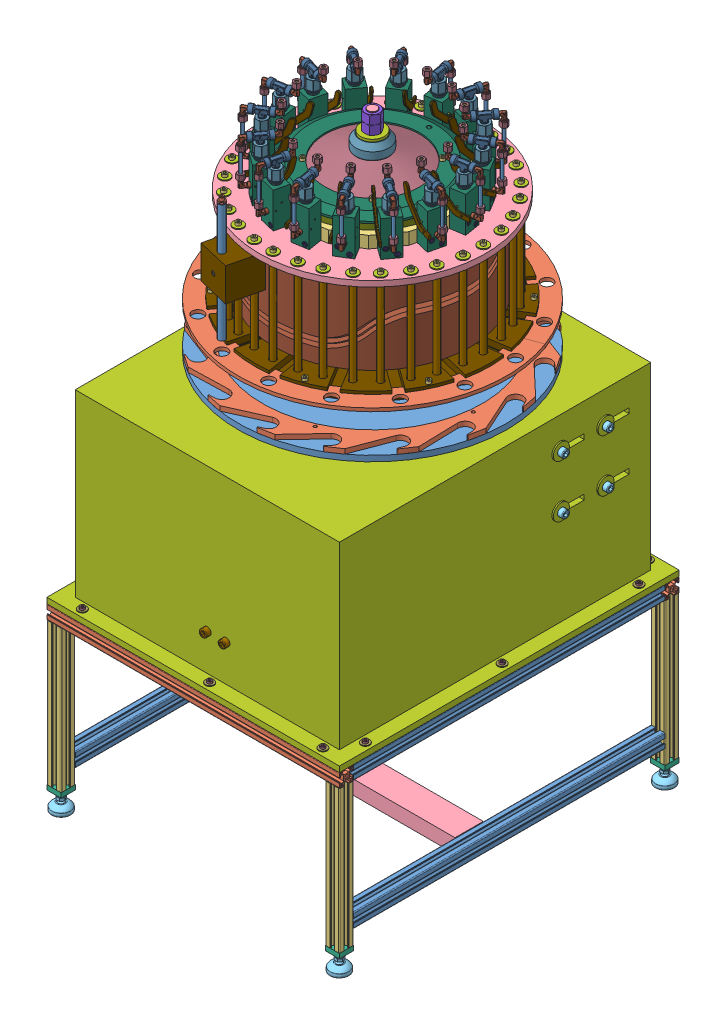
SolidWorks assembly Assieme_FINALE, configuration Default. Lengths in mm.
Overall size (1028.49 1273.72 1028.49).
701 component instances, 77 part files, 51 mates.
Components (placement in the parent):
- SupportoBase_Totale-2: SupportoBase_Totale [Default] at (4.0127 -14.4529 -3.9361) x (0 1 0) z (0 0 1) size (801.2 636.12 736.12)
  - Supporto_base_macchina-1: Supporto_base_macchina [Default] at origin size (378.2 636.12 736.12)
    - profilato_30x30_590-3: profilato_30x30_590 [Default] at (275.414 713.7262 -66.645) size (30 30 660)
    - profilato_30x30_590-5: profilato_30x30_590 [Default] at (275.414 123.7262 -66.645) size (30 30 660)
    - profilato_30x30_550-5: profilato_30x30_550 [Default] at (275.414 703.7262 -716.645) x (1 0 0) z (0 1 0) size (30 30 620)
    - profilato_30x30_550-6: profilato_30x30_550 [Default] at (275.414 703.7262 -26.645) x (1 0 0) z (0 1 0) size (30 30 620)
    - profilato_30x30_272-5: profilato_30x30_272 [Default] at (-16.586 123.7262 -716.645) x (0 0 1) z (-1 0 0) size (30 30 302)
    - profilato_30x30_272-6: profilato_30x30_272 [Default] at (-16.586 713.7262 -716.645) x (0 0 1) z (-1 0 0) size (30 30 302)
    - profilato_30x30_272-7: profilato_30x30_272 [Default] at (235.414 123.7262 -26.645) x (0 0 -1) z (1 0 0) size (30 30 302)
    - profilato_30x30_272-8: profilato_30x30_272 [Default] at (-16.586 713.7262 -26.645) x (0 0 1) z (-1 0 0) size (30 30 302)
    - profilo_U_60x30_490_supporto_base_macchina-1: profilo_U_60x30_490_supporto_base_macchina [Default] at (15.1 707.7262 -323.6583) x (0 0 1) z (0 -1 0) size (60 30 569)
    - profilato_30x30_590-6: profilato_30x30_590 [Default] at (3.414 123.7262 -66.645) size (30 30 660)
    - profilato_30x30_590-7: profilato_30x30_590 [Default] at (3.414 713.7262 -676.645) x (-1 0 0) z (0 0 -1) size (30 30 660)
    - 6322125-1: 6322125 [Default] at (-85.2818 713.7262 -26.645) x (0 0 -1) z (1 0 0) size (40 40 71.2)
    - 6322125-2: 6322125 [Default] at (-85.2818 713.7262 -716.645) x (0 0 -1) z (1 0 0) size (40 40 71.2)
    - 6322125-3: 6322125 [Default] at (-85.2818 123.7262 -26.645) x (0 -0.924225 -0.381849) z (1 0 0) size (40 40 71.2)
    - 6322125-4: 6322125 [Default] at (-85.2818 123.7262 -716.645) x (0 0 -1) z (1 0 0) size (40 40 71.2)
    - tappo_filettato_Supporto_base_macchina-1: tappo_filettato_Supporto_base_macchina [Default] at (-41.586 123.7262 -26.645) x (0 0 1) z (-1 0 0) size (30 30 10.37)
    - tappo_filettato_Supporto_base_macchina-2: tappo_filettato_Supporto_base_macchina [Default] at (-41.586 123.7262 -716.645) x (0 0 1) z (-1 0 0) size (30 30 10.37)
    - tappo_filettato_Supporto_base_macchina-3: tappo_filettato_Supporto_base_macchina [Default] at (-41.586 713.7262 -716.645) x (0 0 1) z (-1 0 0) size (30 30 10.37)
    - tappo_filettato_Supporto_base_macchina-4: tappo_filettato_Supporto_base_macchina [Default] at (-51.586 713.7262 -26.645) x (0 0 -1) z (1 0 0) size (30 30 10.37)
  - assieme_base-1: assieme_base [Default] at (466.8009 1138.7262 -472.0974) x (0 0 -1) z (0 -1 0) size (720 423 620)
    - Supporto di Base per macchina-1: Supporto di Base per macchina [Default] at (-460.4524 -176.3869 1030) size (720 403 620)
    - canotto di supporto-1: canotto di supporto [Default] at (-100.4524 134.8265 740) x (0 1 0) z (-0.866025 0 0.5) size (220 238 238)
    - m10 35mm-7: m10 35mm [ISO 4762 M10 x 35 - 35N] at (4.5476 246.6131 740) x (0 -1 0) z (1 0 0) size (45 16 16)
    - m10 35mm-8: m10 35mm [ISO 4762 M10 x 35 - 35N] at (-47.9524 246.6131 649.0673) x (0 -1 0) z (0.5 0 -0.866025) size (45 16 16)
    - m10 35mm-9: m10 35mm [ISO 4762 M10 x 35 - 35N] at (-152.9524 246.6131 649.0673) x (0 -1 0) z (-0.5 0 -0.866025) size (45 16 16)
    - m10 35mm-10: m10 35mm [ISO 4762 M10 x 35 - 35N] at (-205.4524 246.6131 740) x (0 -1 0) z (-1 0 0) size (45 16 16)
    - m10 35mm-11: m10 35mm [ISO 4762 M10 x 35 - 35N] at (-152.9524 246.6131 830.9327) x (0 -1 0) z (-0.5 0 0.866025) size (45 16 16)
    - m10 35mm-12: m10 35mm [ISO 4762 M10 x 35 - 35N] at (-47.9524 246.6131 830.9327) x (0 -1 0) z (0.5 0 0.866025) size (45 16 16)
    - Traversa di blocco albero-1: Traversa di blocco albero [Default] at (-100.4524 -86.3869 772.5) size (644 42 65)
    - m10 35mm-13: m10 35mm [ISO 4762 M10 x 35 - 35N] at (239.5476 -86.3869 760) x (-1 0 0) z (0 -1 0) size (45 16 16)
    - m10 35mm-16: m10 35mm [ISO 4762 M10 x 35 - 35N] at (239.5476 -86.3869 720) x (-1 0 0) z (0 -1 0) size (45 16 16)
    - m10 35mm-17: m10 35mm [ISO 4762 M10 x 35 - 35N] at (-440.4524 -86.3869 720) x (1 0 0) z (0 1 0) size (45 16 16)
    - m10 35mm-18: m10 35mm [ISO 4762 M10 x 35 - 35N] at (-440.4524 -86.3869 760) x (1 0 0) z (0 1 0) size (45 16 16)
  - DadoT-2: DadoT [Default] at (288.4104 668.7262 -716.645) x (0 0 -1) z (0 -1 0) size (16.5 6 8)
  - DadoT-9: DadoT [Default] at (288.4104 668.7262 -26.645) x (0 0 -1) z (0 -1 0) size (16.5 6 8)
  - DadoT-10: DadoT [Default] at (288.6104 713.7262 -661.645) x (0 1 0) z (0 0 -1) size (16.5 6 8)
  - DadoT-11: DadoT [Default] at (288.6104 713.7262 -371.645) x (0 1 0) z (0 0 -1) size (16.5 6 8)
  - DadoT-12: DadoT [Default] at (288.6104 713.7262 -81.645) x (0 1 0) z (0 0 -1) size (16.5 6 8)
  - DadoT-13: DadoT [Default] at (288.6104 123.7262 -661.645) x (0 1 0) z (0 0 -1) size (16.5 6 8)
  - DadoT-15: DadoT [Default] at (288.6104 123.7262 -371.645) x (0 1 0) z (0 0 -1) size (16.5 6 8)
  - DadoT-17: DadoT [Default] at (288.6104 123.7262 -81.645) x (0 1 0) z (0 0 -1) size (16.5 6 8)
  - RosettaM6-1: RosettaM6 [Washer ISO 7093 - 6] at (302.414 713.7262 -661.645) x (-1 0 0) z (0 0 1) size (1.6 18 18)
  - ViteM6-20-1: ViteM6-20 [ISO 4762 M6 x 20 - 20S] at (308.414 713.7262 -661.645) x (-1 0 0) z (0 0 1) size (26 10 10)
  - RosettaM6-2: RosettaM6 [Washer ISO 7093 - 6] at (302.414 668.7262 -716.645) x (-1 0 0) z (0 0 1) size (1.6 18 18)
  - ViteM6-20-2: ViteM6-20 [ISO 4762 M6 x 20 - 20S] at (308.414 668.7262 -716.645) x (-1 0 0) z (0 0 1) size (26 10 10)
  - RosettaM6-3: RosettaM6 [Washer ISO 7093 - 6] at (302.414 713.7262 -371.645) x (-1 0 0) z (0 0 1) size (1.6 18 18)
  - RosettaM6-4: RosettaM6 [Washer ISO 7093 - 6] at (302.414 713.7262 -81.645) x (-1 0 0) z (0 0 1) size (1.6 18 18)
  - ViteM6-20-3: ViteM6-20 [ISO 4762 M6 x 20 - 20S] at (308.414 713.7262 -371.645) x (-1 0 0) z (0 0 1) size (26 10 10)
  - ViteM6-20-4: ViteM6-20 [ISO 4762 M6 x 20 - 20S] at (308.414 713.7262 -81.645) x (-1 0 0) z (0 0 1) size (26 10 10)
  - RosettaM6-5: RosettaM6 [Washer ISO 7093 - 6] at (302.414 123.7262 -661.645) x (-1 0 0) z (0 0 1) size (1.6 18 18)
  - ViteM6-20-5: ViteM6-20 [ISO 4762 M6 x 20 - 20S] at (308.414 123.7262 -661.645) x (-1 0 0) z (0 0 1) size (26 10 10)
  - RosettaM6-6: RosettaM6 [Washer ISO 7093 - 6] at (302.414 123.7262 -371.645) x (-1 0 0) z (0 0 1) size (1.6 18 18)
  - RosettaM6-7: RosettaM6 [Washer ISO 7093 - 6] at (302.414 123.7262 -81.645) x (-1 0 0) z (0 0 1) size (1.6 18 18)
  - ViteM6-20-6: ViteM6-20 [ISO 4762 M6 x 20 - 20S] at (308.414 123.7262 -371.645) x (-1 0 0) z (0 0 1) size (26 10 10)
  - ViteM6-20-7: ViteM6-20 [ISO 4762 M6 x 20 - 20S] at (308.414 123.7262 -81.645) x (-1 0 0) z (0 0 1) size (26 10 10)
  - ViteM6-20-8: ViteM6-20 [ISO 4762 M6 x 20 - 20S] at (308.414 398.7262 -716.645) x (-1 0 0) z (0 0 1) size (26 10 10)
  - RosettaM6-8: RosettaM6 [Washer ISO 7093 - 6] at (302.414 398.7262 -716.645) x (-1 0 0) z (0 0 1) size (1.6 18 18)
  - DadoT-19: DadoT [Default] at (288.4104 398.7262 -716.645) x (0 0 -1) z (0 -1 0) size (16.5 6 8)
  - DadoT-20: DadoT [Default] at (288.4104 158.7262 -716.645) x (0 0 -1) z (0 -1 0) size (16.5 6 8)
  - RosettaM6-9: RosettaM6 [Washer ISO 7093 - 6] at (302.414 158.7262 -716.645) x (-1 0 0) z (0 0 1) size (1.6 18 18)
  - ViteM6-20-9: ViteM6-20 [ISO 4762 M6 x 20 - 20S] at (308.414 158.7262 -716.645) x (-1 0 0) z (0 0 1) size (26 10 10)
  - DadoT-21: DadoT [Default] at (288.4104 668.7262 -26.645) x (0 0 -1) z (0 -1 0) size (16.5 6 8)
  - RosettaM6-10: RosettaM6 [Washer ISO 7093 - 6] at (302.414 668.7262 -26.645) x (-1 0 0) z (0 0 1) size (1.6 18 18)
  - ViteM6-20-10: ViteM6-20 [ISO 4762 M6 x 20 - 20S] at (308.414 668.7262 -26.645) x (-1 0 0) z (0 0 1) size (26 10 10)
  - DadoT-22: DadoT [Default] at (288.4104 158.7262 -26.645) x (0 0 -1) z (0 -1 0) size (16.5 6 8)
  - RosettaM6-11: RosettaM6 [Washer ISO 7093 - 6] at (302.414 158.7262 -26.645) x (-1 0 0) z (0 0 1) size (1.6 18 18)
  - ViteM6-20-11: ViteM6-20 [ISO 4762 M6 x 20 - 20S] at (308.414 158.7262 -26.645) x (-1 0 0) z (0 0 1) size (26 10 10)
  - ViteM6-20-12: ViteM6-20 [ISO 4762 M6 x 20 - 20S] at (308.414 398.7262 -26.645) x (-1 0 0) z (0 0 1) size (26 10 10)
  - RosettaM6-12: RosettaM6 [Washer ISO 7093 - 6] at (302.414 398.7262 -26.645) x (-1 0 0) z (0 0 1) size (1.6 18 18)
  - DadoT-23: DadoT [Default] at (288.4104 398.7262 -26.645) x (0 0 -1) z (0 -1 0) size (16.5 6 8)
- motoriduttore-1: motoriduttore [Default] at (-164.7135 275.9611 -1137.0941) x (0 0 1) z (-1 0 0) size (200 160 175)
- Assieme_Riduttore-1: Assieme_Riduttore [Default] at (-58.5438 520.923 -522.9431) x (0 1 0) z (-0.993104 0 -0.117237) size (226 168.82 169.04)
  - AlberoRiduttore-1: AlberoRiduttore [Default] at (-61.6906 7.4655 211) size (201 29 29)
  - linguetta_uni6604_b_8x7x50-1: linguetta_uni6604_b_8x7x50 [Default] at (-116.7419 7.4655 226) x (1 0 0) z (0 1 0) size (50 7 8)
  - linguetta_uni6604_b_8x7x35-1: linguetta_uni6604_b_8x7x35 [Default] at (-33.7419 7.4655 226.5) x (1 0 0) z (0 1 0) size (35 7 8)
  - linguetta_uni6604_b_8x7x35-2: linguetta_uni6604_b_8x7x35 [Default] at (41.2581 7.4655 226.5) x (1 0 0) z (0 1 0) size (35 7 8)
  - ASSIEME-LASS-90-VERS-B-O-25-3D.step-1: ASSIEME-LASS-90-VERS-B-O-25-3D.step [Default] at (-111.3519 -70.5563 279.3493) x (-1 0 0) z (0 0.707107 -0.707107) size (64.28 105 105)
  - Rondella di fermo-1: Rondella di fermo [Default] at (-122.7419 7.4655 211) x (0 0.707107 -0.707107) z (-1 0 0) size (36 36 3)
  - M8 25 mm-1: M8 25 mm [ISO 4762 M8 x 25 - 25N] at (92.2581 7.4655 211) x (-1 0 0) z (0 1 0) size (33 13 13)
  - M8 25 mm-2: M8 25 mm [ISO 4762 M8 x 25 - 25N] at (-133.7419 7.4655 211) x (1 0 0) z (0 -0.707107 0.707107) size (33 13 13)
  - M6 16mm-3: M6 16mm [ISO 4762 M6 x 16 - 16N] at (-44.8119 40.5589 196.8286) x (-1 0 0) z (0 0.935687 0.352831) size (22 10 10)
  - M6 16mm-14: M6 16mm [ISO 4762 M6 x 16 - 16N] at (-44.8119 11.7394 175.2546) x (-1 0 0) z (0 0.773404 -0.633913) size (22 10 10)
  - M6 16mm-15: M6 16mm [ISO 4762 M6 x 16 - 16N] at (-44.8119 -21.354 189.426) x (-1 0 0) z (0 -0.162283 -0.986744) size (22 10 10)
  - M6 16mm-16: M6 16mm [ISO 4762 M6 x 16 - 16N] at (-44.8119 -25.6279 225.1714) x (-1 0 0) z (0 -0.935687 -0.352831) size (22 10 10)
  - M6 16mm-17: M6 16mm [ISO 4762 M6 x 16 - 16N] at (-44.8119 3.1916 246.7454) x (-1 0 0) z (0 -0.773404 0.633913) size (22 10 10)
  - M6 16mm-18: M6 16mm [ISO 4762 M6 x 16 - 16N] at (-44.8119 36.285 232.574) x (-1 0 0) z (0 0.162283 0.986744) size (22 10 10)
  - Parte1^Assieme_Riduttore-1: Parte1^Assieme_Riduttore [Default] at origin (virtual)
  - ruota dentata m22-4: ruota dentata m22 [Chain wheel ISO - 22Z 10A-1 --22SA36.0N] at (-59.7419 7.4655 211) x (1 0 0) z (0 -0.599278 0.800541) size (8.93 120.13 121.23)
  - Rondella di fermo-2: Rondella di fermo [Default] at (84.2581 7.4655 211) x (0 0 1) z (-1 0 0) size (36 36 3)
- M10 50mm-1: M10 50mm [ISO 4762 M10 x 50 - 50N] at (-121.7135 603.4611 -513.0941) x (-1 0 0) z (0 -0.924225 -0.381849) size (60 16 16)
- M10 50mm-2: M10 50mm [ISO 4762 M10 x 50 - 50N] at (-121.7135 492.4611 -513.0941) x (-1 0 0) z (0 0 1) size (60 16 16)
- M10 50mm-5: M10 50mm [ISO 4762 M10 x 50 - 50N] at (-121.7135 603.4611 -608.0941) x (-1 0 0) z (0 0 1) size (60 16 16)
- M10 50mm-4: M10 50mm [ISO 4762 M10 x 50 - 50N] at (-121.7135 492.4611 -608.0941) x (-1 0 0) z (0 0 1) size (60 16 16)
- dado M10-13: dado M10 [ISO - 4033 - M10 - W - N] at (-174.0135 603.4611 -608.0941) x (0 0 1) z (-1 0 0) size (16 18.48 9.3)
- dado M10-14: dado M10 [ISO - 4033 - M10 - W - N] at (-174.0135 603.4611 -513.0941) x (0 0 1) z (-1 0 0) size (16 18.48 9.3)
- dado M10-16: dado M10 [ISO - 4033 - M10 - W - N] at (-174.0135 492.4611 -608.0941) x (0 0 1) z (-1 0 0) size (16 18.48 9.3)
- dado M10-15: dado M10 [ISO - 4033 - M10 - W - N] at (-174.0135 492.4611 -513.0941) x (0 0 1) z (-1 0 0) size (16 18.48 9.3)
- rondella large-16: rondella large [Washer ISO 7094 - 10] at (-134.7135 603.4611 -513.0941) x (-1 0 0) z (0 0.924225 0.381849) size (3 34 34)
- rondella large-15: rondella large [Washer ISO 7094 - 10] at (-134.7135 492.4611 -513.0941) x (-1 0 0) z (0 0 1) size (3 34 34)
- rondella large-17: rondella large [Washer ISO 7094 - 10] at (-134.7135 492.4611 -608.0941) x (-1 0 0) z (0 0 1) size (3 34 34)
- rondella large-14: rondella large [Washer ISO 7094 - 10] at (-134.7135 603.4611 -608.0941) x (-1 0 0) z (0 0 1) size (3 34 34)
- catena_maschio-1: catena_maschio [Default] at (-321.9473 463.4961 -580.6395) x (-0.810007 0 0.58642) z (0 1 0) size (28.67 12.73 20.3)
- catena_femmina-1: catena_femmina [Default] at (-334.299 463.4961 -567.4631) x (0.810007 0 -0.58642) z (0 1 0) size (30.04 14.2 13.87)
  - ansi_50_02-1: ansi_50_02 [Default] at (17.7318 3.4296 0) x (1 0 0) z (0 0 -1) size (30.04 14.2 13.87)
  - ansi_50_03-1: ansi_50_03 [Default] at (17.7318 3.4296 -0.11) x (1 0 0) z (0 0 -1) size (10.16 10.16 9.46)
  - ansi_50_04-1: ansi_50_04 [Default] at (17.7318 3.4296 0.11) x (1 0 0) z (0 0 -1) size (10.16 10.16 9.46)
- rondella M8-3: rondella M8 [ISO 10673-9.3-S] at (-394.7135 376.9611 -360.5811) x (0 -1 0) z (-1 0 0) size (2 18 18)
- rondella M8-4: rondella M8 [ISO 10673-9.3-S] at (-394.7135 376.9611 -390.5811) x (0 -1 0) z (-1 0 0) size (2 18 18)
- M8 25 mm-1: M8 25 mm [ISO 4762 M8 x 25 - 25N] at (-394.7135 368.9611 -390.5811) x (0 1 0) z (0.5 0 0.866025) size (33 13 13)
- M8 25 mm-2: M8 25 mm [ISO 4762 M8 x 25 - 25N] at (-394.7135 366.9611 -360.5811) x (0 1 0) z (-0.5 0 -0.866025) size (33 13 13)
- assieme parte rotante-2: assieme parte rotante [Default] at (-8.3038 623.9178 -528.0599) x (0 1 0) z (-0.913062 0 0.407822) size (749.63 778.63 778.63)
  - albero rotazione piatti-1: albero rotazione piatti [Default] at (60.413 18.3637 415) size (415 200 200)
  - seger 100mm-2: seger 100mm [KS 1336 E - 100] at (-146.4567 18.3637 415) x (0 0 -1) z (1 0 0) size (107.55 112.98 3)
  - SKF - 6020 - 20,DE,NC,20_68-1: SKF - 6020 - 20,DE,NC,20_68 [SKF - 6020 - 20,DE,NC,20_68] at (-131.4567 18.3637 415) x (1 0 0) z (0 -0.434476 -0.900684) size (24 150 150)
  - calettatore d95-1: calettatore d95 [Default] at (-173.8867 18.3637 415) size (39.5 135 135)
  - Chain wheel ISO - 50Z 10A-1-1: Chain wheel ISO - 50Z 10A-1 [Chain wheel ISO - 50Z 10A-1 --50SB120H25L95.0N] at (-164.8867 18.3637 415) size (28.93 262.06 262.51)
  - Disco supporto montaggio e Colonne-1: Disco supporto montaggio e Colonne [Default] at (204.0433 18.3637 415) x (0 -0.866025 -0.5) z (1 0 0) size (499.6 499.6 29)
  - SKF - 6020 - 20,DE,NC,20_68-2: SKF - 6020 - 20,DE,NC,20_68 [SKF - 6020 - 20,DE,NC,20_68] at (62.0433 18.3637 415) x (1 0 0) z (0 -0.432628 -0.901573) size (24 150 150)
  - piatto rotante porta tappi-1: piatto rotante porta tappi [Default] at (99.0433 18.3637 415) x (0 0 -1) z (1 0 0) size (570 570 20.57)
  - disco trasportatore tappi 31-1: disco trasportatore tappi 31 [Default] at (111.0433 18.3637 415) x (0 0.5 -0.866025) z (1 0 0) size (570 570 10.42)
  - Distributore Rotante-1: Distributore Rotante [Default] at (425.0433 18.3637 415) x (0 0.130526 -0.991445) z (1 0 0) size (310 310 25.54)
  - disco trascinato porta distributore vuoto-1: disco trascinato porta distributore vuoto [Default] at (400.0433 18.3637 415) x (0 -0.130526 0.991445) z (-1 0 0) size (480 480 50)
  - m12 35mm-1: m12 35mm [ISO 4762 M12 x 35 - 35N] at (376.0433 -45.1046 366.2991) x (1 0 0) z (0 -0.5 0.866025) size (47 18 18)
  - m12 90mm-3: m12 90mm [ISO 4762 M12 x 90 - 90N] at (203.0433 -21.6363 345.718) x (-1 0 0) z (0 -0.5 0.866025) size (102 18 18)
  - rondella M6-90: rondella M6 [Washer ISO 7094 - 6] at (99.0433 -101.6363 207.1539) x (1 0 0) z (0 -1 0) size (2 22 22)
  - M6 20mm-1: M6 20mm [ISO 4762 M6 x 20 - 20N] at (91.0433 -101.6363 207.1539) x (1 0 0) z (0 0.5 0.866025) size (26 10 10)
  - m12 35mm-2: m12 35mm [ISO 4762 M12 x 35 - 35N] at (376.0433 28.8058 335.6844) x (1 0 0) z (0 -1 0) size (47 18 18)
  - m12 35mm-3: m12 35mm [ISO 4762 M12 x 35 - 35N] at (376.0433 92.2741 384.3853) x (1 0 0) z (0 -0.5 -0.866025) size (47 18 18)
  - m12 35mm-4: m12 35mm [ISO 4762 M12 x 35 - 35N] at (376.0433 81.832 463.7009) x (1 0 0) z (0 0.5 -0.866025) size (47 18 18)
  - m12 35mm-5: m12 35mm [ISO 4762 M12 x 35 - 35N] at (376.0433 7.9216 494.3156) x (1 0 0) z (0 1 0) size (47 18 18)
  - m12 35mm-6: m12 35mm [ISO 4762 M12 x 35 - 35N] at (376.0433 -55.5467 445.6147) x (1 0 0) z (0 0.5 0.866025) size (47 18 18)
  - rondella M6-91: rondella M6 [Washer ISO 7094 - 6] at (99.0433 138.3637 207.1539) x (1 0 0) z (0 -0.5 -0.866025) size (2 22 22)
  - rondella M6-92: rondella M6 [Washer ISO 7094 - 6] at (99.0433 258.3637 415) x (1 0 0) z (0 0.5 -0.866025) size (2 22 22)
  - rondella M6-93: rondella M6 [Washer ISO 7094 - 6] at (99.0433 138.3637 622.8461) x (1 0 0) z (0 1 0) size (2 22 22)
  - rondella M6-94: rondella M6 [Washer ISO 7094 - 6] at (99.0433 -101.6363 622.8461) x (1 0 0) z (0 0.5 0.866025) size (2 22 22)
  - rondella M6-95: rondella M6 [Washer ISO 7094 - 6] at (99.0433 -221.6363 415) x (1 0 0) z (0 -0.5 0.866025) size (2 22 22)
  - M6 20mm-2: M6 20mm [ISO 4762 M6 x 20 - 20N] at (91.0433 138.3637 207.1539) x (1 0 0) z (0 -0.5 0.866025) size (26 10 10)
  - M6 20mm-3: M6 20mm [ISO 4762 M6 x 20 - 20N] at (91.0433 258.3637 415) x (1 0 0) z (0 -1 0) size (26 10 10)
  - M6 20mm-4: M6 20mm [ISO 4762 M6 x 20 - 20N] at (91.0433 138.3637 622.8461) x (1 0 0) z (0 -0.5 -0.866025) size (26 10 10)
  - M6 20mm-5: M6 20mm [ISO 4762 M6 x 20 - 20N] at (91.0433 -101.6363 622.8461) x (1 0 0) z (0 0.5 -0.866025) size (26 10 10)
  - M6 20mm-6: M6 20mm [ISO 4762 M6 x 20 - 20N] at (91.0433 -221.6363 415) x (1 0 0) z (0 1 0) size (26 10 10)
  - m12 90mm-4: m12 90mm [ISO 4762 M12 x 90 - 90N] at (203.0433 58.3637 345.718) x (-1 0 0) z (0 -1 0) size (102 18 18)
  - m12 90mm-5: m12 90mm [ISO 4762 M12 x 90 - 90N] at (203.0433 98.3637 415) x (-1 0 0) z (0 -0.5 -0.866025) size (102 18 18)
  - m12 90mm-6: m12 90mm [ISO 4762 M12 x 90 - 90N] at (203.0433 58.3637 484.282) x (-1 0 0) z (0 0.5 -0.866025) size (102 18 18)
  - m12 90mm-7: m12 90mm [ISO 4762 M12 x 90 - 90N] at (203.0433 -21.6363 484.282) x (-1 0 0) z (0 1 0) size (102 18 18)
  - m12 90mm-8: m12 90mm [ISO 4762 M12 x 90 - 90N] at (203.0433 -61.6363 415) x (-1 0 0) z (0 0.5 0.866025) size (102 18 18)
  - asta scorrimento carello-1: asta scorrimento carello [Default] at (287.5433 70.1437 197.9013) x (0 0 -1) z (1 0 0) size (12 12 225)
  - rondella M6-74: rondella M6 [Washer ISO 7094 - 6] at (175.0433 70.1437 197.9013) x (1 0 0) z (0 -1 0) size (2 22 22)
  - M6 16mm-1: M6 16mm [ISO 4762 M6 x 16 - 16N] at (167.0433 70.1437 197.9013) size (22 10 10)
  - M6 16mm-2: M6 16mm [ISO 4762 M6 x 16 - 16N] at (408.0433 70.1437 197.9013) x (-1 0 0) z (0 0 -1) size (22 10 10)
  - rondella M6-96: rondella M6 [Washer ISO 7094 - 6] at (400.0433 70.1437 197.9013) x (-1 0 0) z (0 1 0) size (2 22 22)
  - rondella M6-112: rondella M6 [Washer ISO 7094 - 6] at (175.0433 24.5373 191.8971) x (1 0 0) z (0 -0.965926 -0.258819) size (2 22 22)
  - M6 16mm-3: M6 16mm [ISO 4762 M6 x 16 - 16N] at (167.0433 24.5373 191.8971) x (1 0 0) z (0 0.258819 -0.965926) size (22 10 10)
  - asta scorrimento carello-2: asta scorrimento carello [Default] at (287.5433 24.5373 191.8971) x (0 0.258819 -0.965926) z (-1 0 0) size (12 12 225)
  - rondella M6-128: rondella M6 [Washer ISO 7094 - 6] at (400.0433 24.5373 191.8971) x (-1 0 0) z (0 0.965926 0.258819) size (2 22 22)
  - M6 16mm-4: M6 16mm [ISO 4762 M6 x 16 - 16N] at (408.0433 24.5373 191.8971) x (-1 0 0) z (0 -0.258819 0.965926) size (22 10 10)
  - AssiemeValvola-1: AssiemeValvola [Default] at (515.3257 103.3637 267.7757) x (0 -0.5 0.866025) z (0 0.866025 0.5) size (90.26 138.63 38)
    - RaccordoT-1: RaccordoT [Default] at origin size (43 29.75 16.5)
    - Raccordo a L-1: Raccordo a L [Default] at (-30 0 0) x (0 -1 0) z (0 0 -1) size (28.34 25.51 14.01)
      - 1809_06_10_01-1: 1809_06_10_01 [Default] at origin size (22.49 23 10)
      - 1809_06_10_02-1: 1809_06_10_02 [Default] at origin size (6.5 8.5 8.5)
      - 1809_06_10_03-1: 1809_06_10_03 [Default] at origin size (11.02 15.01 14.01)
    - Raccordo a L-2: Raccordo a L [Default] at (30 0 0) x (0 1 0) z (0 0 -1) size (28.34 25.51 14.01)
      - 1809_06_10_01-1: 1809_06_10_01 [Default] at origin size (22.49 23 10)
      - 1809_06_10_02-1: 1809_06_10_02 [Default] at origin size (6.5 8.5 8.5)
      - 1809_06_10_03-1: 1809_06_10_03 [Default] at origin size (11.02 15.01 14.01)
    - TappoChiusura-1: TappoChiusura [Default] at (0 -32 0) x (0 -1 0) z (0 0 1) size (38.28 26.74 26.74)
    - CorpoValvola-1: CorpoValvola [Default] at (-15 -115.2824 0) size (30 75 34)
    - Raccordo a L-3: Raccordo a L [Default] at (-30 -88.2824 0) x (0 1 0) z (0 0 1) size (28.34 25.51 14.01)
      - 1809_06_10_01-1: 1809_06_10_01 [Default] at origin size (22.49 23 10)
      - 1809_06_10_02-1: 1809_06_10_02 [Default] at origin size (6.5 8.5 8.5)
      - 1809_06_10_03-1: 1809_06_10_03 [Default] at origin size (11.02 15.01 14.01)
    - Spina_3x38-1: Spina_3x38 [Default] at (0 -68.2824 -21) x (-1 0 0) z (0 0 1) size (3 3 38)
    - Spina_3x38-2: Spina_3x38 [Default] at (-10 -80.2824 -21) x (0.996193 0.087174 0) z (0 0 1) size (3 3 38)
    - M5 40mm-3: M5 40mm [ISO 4762 M5 x 40 - 40N] at (-14.6 -108.7824 9) size (45 8.5 8.5)
    - M5 40mm-2: M5 40mm [ISO 4762 M5 x 40 - 40N] at (-14.6 -96.7824 -9) size (45 8.5 8.5)
    - LevaValvola-1: LevaValvola [Default] at (-24.507 -86.571 -17) x (0.996193 0.087174 0) z (0 0 1) size (77.55 60.2 4)
    - Tubo-1: Tubo [Default] at (-30 -15.9665 0) x (1 0 0) z (0 -1 0) size (6 6 56.4)
  - M6 16mm-5: M6 16mm [ISO 4762 M6 x 16 - 16N] at (167.0433 -16.8778 194.6116) x (1 0 0) z (0 0.382683 0.92388) size (22 10 10)
  - M6 16mm-6: M6 16mm [ISO 4762 M6 x 16 - 16N] at (167.0433 -98.5342 224.874) x (1 0 0) z (0 0.707107 0.707107) size (22 10 10)
  - M6 16mm-7: M6 16mm [ISO 4762 M6 x 16 - 16N] at (167.0433 -162.3939 284.0814) x (1 0 0) z (0 0.92388 0.382683) size (22 10 10)
  - M6 16mm-8: M6 16mm [ISO 4762 M6 x 16 - 16N] at (167.0433 -198.735 363.22) x (1 0 0) z (0 1 0) size (22 10 10)
  - M6 16mm-9: M6 16mm [ISO 4762 M6 x 16 - 16N] at (167.0433 -202.0247 450.2415) x (1 0 0) z (0 0.92388 -0.382683) size (22 10 10)
  - M6 16mm-10: M6 16mm [ISO 4762 M6 x 16 - 16N] at (167.0433 -171.7623 531.8979) x (1 0 0) z (0 0.707107 -0.707107) size (22 10 10)
  - M6 16mm-11: M6 16mm [ISO 4762 M6 x 16 - 16N] at (167.0433 -112.5549 595.7576) x (1 0 0) z (0 0.382683 -0.92388) size (22 10 10)
  - M6 16mm-12: M6 16mm [ISO 4762 M6 x 16 - 16N] at (167.0433 -33.4163 632.0987) x (1 0 0) z (0 0 -1) size (22 10 10)
  - M6 16mm-13: M6 16mm [ISO 4762 M6 x 16 - 16N] at (167.0433 53.6052 635.3884) x (1 0 0) z (0 -0.382683 -0.92388) size (22 10 10)
  - M6 16mm-14: M6 16mm [ISO 4762 M6 x 16 - 16N] at (167.0433 135.2616 605.126) x (1 0 0) z (0 -0.707107 -0.707107) size (22 10 10)
  - M6 16mm-15: M6 16mm [ISO 4762 M6 x 16 - 16N] at (167.0433 199.1213 545.9186) x (1 0 0) z (0 -0.92388 -0.382683) size (22 10 10)
  - M6 16mm-16: M6 16mm [ISO 4762 M6 x 16 - 16N] at (167.0433 235.4624 466.78) x (1 0 0) z (0 -1 0) size (22 10 10)
  - M6 16mm-17: M6 16mm [ISO 4762 M6 x 16 - 16N] at (167.0433 238.7521 379.7585) x (1 0 0) z (0 -0.92388 0.382683) size (22 10 10)
  - M6 16mm-18: M6 16mm [ISO 4762 M6 x 16 - 16N] at (167.0433 208.4897 298.1021) x (1 0 0) z (0 -0.707107 0.707107) size (22 10 10)
  - M6 16mm-19: M6 16mm [ISO 4762 M6 x 16 - 16N] at (167.0433 149.2823 234.2424) x (1 0 0) z (0 -0.382683 0.92388) size (22 10 10)
  - rondella M6-75: rondella M6 [Washer ISO 7094 - 6] at (175.0433 -16.8778 194.6116) x (1 0 0) z (0 -0.92388 0.382683) size (2 22 22)
  - rondella M6-76: rondella M6 [Washer ISO 7094 - 6] at (175.0433 -98.5342 224.874) x (1 0 0) z (0 -0.707107 0.707107) size (2 22 22)
  - rondella M6-77: rondella M6 [Washer ISO 7094 - 6] at (175.0433 -162.3939 284.0814) x (1 0 0) z (0 -0.382683 0.92388) size (2 22 22)
  - rondella M6-78: rondella M6 [Washer ISO 7094 - 6] at (175.0433 -198.735 363.22) size (2 22 22)
  - rondella M6-79: rondella M6 [Washer ISO 7094 - 6] at (175.0433 -202.0247 450.2415) x (1 0 0) z (0 0.382683 0.92388) size (2 22 22)
  - rondella M6-80: rondella M6 [Washer ISO 7094 - 6] at (175.0433 -171.7623 531.8979) x (1 0 0) z (0 0.707107 0.707107) size (2 22 22)
  - rondella M6-81: rondella M6 [Washer ISO 7094 - 6] at (175.0433 -112.5549 595.7576) x (1 0 0) z (0 0.92388 0.382683) size (2 22 22)
  - rondella M6-82: rondella M6 [Washer ISO 7094 - 6] at (175.0433 -33.4163 632.0987) x (1 0 0) z (0 1 0) size (2 22 22)
  - rondella M6-83: rondella M6 [Washer ISO 7094 - 6] at (175.0433 53.6052 635.3884) x (1 0 0) z (0 0.92388 -0.382683) size (2 22 22)
  - rondella M6-84: rondella M6 [Washer ISO 7094 - 6] at (175.0433 135.2616 605.126) x (1 0 0) z (0 0.707107 -0.707107) size (2 22 22)
  - rondella M6-85: rondella M6 [Washer ISO 7094 - 6] at (175.0433 199.1213 545.9186) x (1 0 0) z (0 0.382683 -0.92388) size (2 22 22)
  - rondella M6-86: rondella M6 [Washer ISO 7094 - 6] at (175.0433 235.4624 466.78) x (1 0 0) z (0 0 -1) size (2 22 22)
  - rondella M6-87: rondella M6 [Washer ISO 7094 - 6] at (175.0433 238.7521 379.7585) x (1 0 0) z (0 -0.382683 -0.92388) size (2 22 22)
  - rondella M6-88: rondella M6 [Washer ISO 7094 - 6] at (175.0433 208.4897 298.1021) x (1 0 0) z (0 -0.707107 -0.707107) size (2 22 22)
  - rondella M6-89: rondella M6 [Washer ISO 7094 - 6] at (175.0433 149.2823 234.2424) x (1 0 0) z (0 -0.92388 -0.382683) size (2 22 22)
  - asta scorrimento carello-3: asta scorrimento carello [Default] at (287.5433 -16.8778 194.6116) x (0 -0.382683 -0.92388) z (1 0 0) size (12 12 225)
  - asta scorrimento carello-4: asta scorrimento carello [Default] at (287.5433 -98.5342 224.874) x (0 -0.707107 -0.707107) z (1 0 0) size (12 12 225)
  - asta scorrimento carello-5: asta scorrimento carello [Default] at (287.5433 -162.3939 284.0814) x (0 -0.92388 -0.382683) z (1 0 0) size (12 12 225)
  - asta scorrimento carello-6: asta scorrimento carello [Default] at (287.5433 -198.735 363.22) x (0 -1 0) z (1 0 0) size (12 12 225)
  - asta scorrimento carello-7: asta scorrimento carello [Default] at (287.5433 -202.0247 450.2415) x (0 -0.92388 0.382683) z (1 0 0) size (12 12 225)
  - asta scorrimento carello-8: asta scorrimento carello [Default] at (287.5433 -171.7623 531.8979) x (0 -0.707107 0.707107) z (1 0 0) size (12 12 225)
  - asta scorrimento carello-9: asta scorrimento carello [Default] at (287.5433 -112.5549 595.7576) x (0 -0.382683 0.92388) z (1 0 0) size (12 12 225)
  - asta scorrimento carello-10: asta scorrimento carello [Default] at (287.5433 -33.4163 632.0987) x (0 0 1) z (1 0 0) size (12 12 225)
  - asta scorrimento carello-11: asta scorrimento carello [Default] at (287.5433 53.6052 635.3884) x (0 0.382683 0.92388) z (1 0 0) size (12 12 225)
  - asta scorrimento carello-12: asta scorrimento carello [Default] at (287.5433 135.2616 605.126) x (0 0.707107 0.707107) z (1 0 0) size (12 12 225)
  - asta scorrimento carello-13: asta scorrimento carello [Default] at (287.5433 199.1213 545.9186) x (0 0.92388 0.382683) z (1 0 0) size (12 12 225)
  - asta scorrimento carello-14: asta scorrimento carello [Default] at (287.5433 235.4624 466.78) x (0 1 0) z (1 0 0) size (12 12 225)
  - asta scorrimento carello-15: asta scorrimento carello [Default] at (287.5433 238.7521 379.7585) x (0 0.92388 -0.382683) z (1 0 0) size (12 12 225)
  - asta scorrimento carello-16: asta scorrimento carello [Default] at (287.5433 208.4897 298.1021) x (0 0.707107 -0.707107) z (1 0 0) size (12 12 225)
  - asta scorrimento carello-17: asta scorrimento carello [Default] at (287.5433 149.2823 234.2424) x (0 0.382683 -0.92388) z (1 0 0) size (12 12 225)
  - M6 16mm-20: M6 16mm [ISO 4762 M6 x 16 - 16N] at (408.0433 -16.8778 194.6116) x (-1 0 0) z (0 -0.382683 -0.92388) size (22 10 10)
  - M6 16mm-21: M6 16mm [ISO 4762 M6 x 16 - 16N] at (408.0433 -98.5342 224.874) x (-1 0 0) z (0 -0.707107 -0.707107) size (22 10 10)
  - M6 16mm-22: M6 16mm [ISO 4762 M6 x 16 - 16N] at (408.0433 -162.3939 284.0814) x (-1 0 0) z (0 -0.92388 -0.382683) size (22 10 10)
  - M6 16mm-23: M6 16mm [ISO 4762 M6 x 16 - 16N] at (408.0433 -198.735 363.22) x (-1 0 0) z (0 -1 0) size (22 10 10)
  - M6 16mm-24: M6 16mm [ISO 4762 M6 x 16 - 16N] at (408.0433 -202.0247 450.2415) x (-1 0 0) z (0 -0.92388 0.382683) size (22 10 10)
  - M6 16mm-25: M6 16mm [ISO 4762 M6 x 16 - 16N] at (408.0433 -171.7623 531.8979) x (-1 0 0) z (0 -0.707107 0.707107) size (22 10 10)
  - M6 16mm-26: M6 16mm [ISO 4762 M6 x 16 - 16N] at (408.0433 -112.5549 595.7576) x (-1 0 0) z (0 -0.382683 0.92388) size (22 10 10)
  - M6 16mm-27: M6 16mm [ISO 4762 M6 x 16 - 16N] at (408.0433 -33.4163 632.0987) x (-1 0 0) z (0 0 1) size (22 10 10)
  - M6 16mm-28: M6 16mm [ISO 4762 M6 x 16 - 16N] at (408.0433 53.6052 635.3884) x (-1 0 0) z (0 0.382683 0.92388) size (22 10 10)
  - M6 16mm-29: M6 16mm [ISO 4762 M6 x 16 - 16N] at (408.0433 135.2616 605.126) x (-1 0 0) z (0 0.707107 0.707107) size (22 10 10)
  - M6 16mm-30: M6 16mm [ISO 4762 M6 x 16 - 16N] at (408.0433 199.1213 545.9186) x (-1 0 0) z (0 0.92388 0.382683) size (22 10 10)
  - M6 16mm-31: M6 16mm [ISO 4762 M6 x 16 - 16N] at (408.0433 235.4624 466.78) x (-1 0 0) z (0 1 0) size (22 10 10)
  - M6 16mm-32: M6 16mm [ISO 4762 M6 x 16 - 16N] at (408.0433 238.7521 379.7585) x (-1 0 0) z (0 0.92388 -0.382683) size (22 10 10)
  - M6 16mm-33: M6 16mm [ISO 4762 M6 x 16 - 16N] at (408.0433 208.4897 298.1021) x (-1 0 0) z (0 0.707107 -0.707107) size (22 10 10)
  - M6 16mm-34: M6 16mm [ISO 4762 M6 x 16 - 16N] at (408.0433 149.2823 234.2424) x (-1 0 0) z (0 0.382683 -0.92388) size (22 10 10)
  - rondella M6-97: rondella M6 [Washer ISO 7094 - 6] at (400.0433 -16.8778 194.6116) x (-1 0 0) z (0 0.92388 -0.382683) size (2 22 22)
  - rondella M6-98: rondella M6 [Washer ISO 7094 - 6] at (400.0433 -98.5342 224.874) x (-1 0 0) z (0 0.707107 -0.707107) size (2 22 22)
  - rondella M6-99: rondella M6 [Washer ISO 7094 - 6] at (400.0433 -162.3939 284.0814) x (-1 0 0) z (0 0.382683 -0.92388) size (2 22 22)
  - rondella M6-100: rondella M6 [Washer ISO 7094 - 6] at (400.0433 -198.735 363.22) x (-1 0 0) z (0 0 -1) size (2 22 22)
  - rondella M6-101: rondella M6 [Washer ISO 7094 - 6] at (400.0433 -202.0247 450.2415) x (-1 0 0) z (0 -0.382683 -0.92388) size (2 22 22)
  - rondella M6-102: rondella M6 [Washer ISO 7094 - 6] at (400.0433 -171.7623 531.8979) x (-1 0 0) z (0 -0.707107 -0.707107) size (2 22 22)
  - rondella M6-103: rondella M6 [Washer ISO 7094 - 6] at (400.0433 -112.5549 595.7576) x (-1 0 0) z (0 -0.92388 -0.382683) size (2 22 22)
  - rondella M6-104: rondella M6 [Washer ISO 7094 - 6] at (400.0433 -33.4163 632.0987) x (-1 0 0) z (0 -1 0) size (2 22 22)
  - rondella M6-105: rondella M6 [Washer ISO 7094 - 6] at (400.0433 53.6052 635.3884) x (-1 0 0) z (0 -0.92388 0.382683) size (2 22 22)
  - rondella M6-106: rondella M6 [Washer ISO 7094 - 6] at (400.0433 135.2616 605.126) x (-1 0 0) z (0 -0.707107 0.707107) size (2 22 22)
  - rondella M6-107: rondella M6 [Washer ISO 7094 - 6] at (400.0433 199.1213 545.9186) x (-1 0 0) z (0 -0.382683 0.92388) size (2 22 22)
  - rondella M6-108: rondella M6 [Washer ISO 7094 - 6] at (400.0433 235.4624 466.78) x (-1 0 0) z (0 0 1) size (2 22 22)
  - rondella M6-109: rondella M6 [Washer ISO 7094 - 6] at (400.0433 238.7521 379.7585) x (-1 0 0) z (0 0.382683 0.92388) size (2 22 22)
  - rondella M6-110: rondella M6 [Washer ISO 7094 - 6] at (400.0433 208.4897 298.1021) x (-1 0 0) z (0 0.707107 0.707107) size (2 22 22)
  - rondella M6-111: rondella M6 [Washer ISO 7094 - 6] at (400.0433 149.2823 234.2424) x (-1 0 0) z (0 0.92388 0.382683) size (2 22 22)
  - rondella M6-113: rondella M6 [Washer ISO 7094 - 6] at (175.0433 -61.3104 206.5173) x (1 0 0) z (0 -0.991445 0.130526) size (2 22 22)
  - rondella M6-114: rondella M6 [Washer ISO 7094 - 6] at (175.0433 -135.0285 252.8771) x (1 0 0) z (0 -0.866025 0.5) size (2 22 22)
  - rondella M6-115: rondella M6 [Washer ISO 7094 - 6] at (175.0433 -185.3939 323.9186) x (1 0 0) z (0 -0.608761 0.793353) size (2 22 22)
  - rondella M6-116: rondella M6 [Washer ISO 7094 - 6] at (175.0433 -204.7392 408.8264) x (1 0 0) z (0 -0.258819 0.965926) size (2 22 22)
  - rondella M6-117: rondella M6 [Washer ISO 7094 - 6] at (175.0433 -190.119 494.6741) x (1 0 0) z (0 0.130526 0.991445) size (2 22 22)
  - rondella M6-118: rondella M6 [Washer ISO 7094 - 6] at (175.0433 -143.7592 568.3922) x (1 0 0) z (0 0.5 0.866025) size (2 22 22)
  - rondella M6-119: rondella M6 [Washer ISO 7094 - 6] at (175.0433 -72.7177 618.7576) x (1 0 0) z (0 0.793353 0.608761) size (2 22 22)
  - rondella M6-120: rondella M6 [Washer ISO 7094 - 6] at (175.0433 12.1901 638.1029) x (1 0 0) z (0 0.965926 0.258819) size (2 22 22)
  - rondella M6-121: rondella M6 [Washer ISO 7094 - 6] at (175.0433 98.0378 623.4827) x (1 0 0) z (0 0.991445 -0.130526) size (2 22 22)
  - rondella M6-122: rondella M6 [Washer ISO 7094 - 6] at (175.0433 171.7559 577.1229) x (1 0 0) z (0 0.866025 -0.5) size (2 22 22)
  - rondella M6-123: rondella M6 [Washer ISO 7094 - 6] at (175.0433 222.1213 506.0814) x (1 0 0) z (0 0.608761 -0.793353) size (2 22 22)
  - rondella M6-124: rondella M6 [Washer ISO 7094 - 6] at (175.0433 241.4666 421.1736) x (1 0 0) z (0 0.258819 -0.965926) size (2 22 22)
  - rondella M6-125: rondella M6 [Washer ISO 7094 - 6] at (175.0433 226.8464 335.3259) x (1 0 0) z (0 -0.130526 -0.991445) size (2 22 22)
  - rondella M6-126: rondella M6 [Washer ISO 7094 - 6] at (175.0433 180.4866 261.6078) x (1 0 0) z (0 -0.5 -0.866025) size (2 22 22)
  - rondella M6-127: rondella M6 [Washer ISO 7094 - 6] at (175.0433 109.4451 211.2424) x (1 0 0) z (0 -0.793353 -0.608761) size (2 22 22)
  - M6 16mm-35: M6 16mm [ISO 4762 M6 x 16 - 16N] at (167.0433 -61.3104 206.5173) x (1 0 0) z (0 -0.130526 -0.991445) size (22 10 10)
  - M6 16mm-36: M6 16mm [ISO 4762 M6 x 16 - 16N] at (167.0433 -135.0285 252.8771) x (1 0 0) z (0 -0.5 -0.866025) size (22 10 10)
  - M6 16mm-37: M6 16mm [ISO 4762 M6 x 16 - 16N] at (167.0433 -185.3939 323.9186) x (1 0 0) z (0 -0.793353 -0.608761) size (22 10 10)
  - M6 16mm-38: M6 16mm [ISO 4762 M6 x 16 - 16N] at (167.0433 -204.7392 408.8264) x (1 0 0) z (0 -0.965926 -0.258819) size (22 10 10)
  - M6 16mm-39: M6 16mm [ISO 4762 M6 x 16 - 16N] at (167.0433 -190.119 494.6741) x (1 0 0) z (0 -0.991445 0.130526) size (22 10 10)
